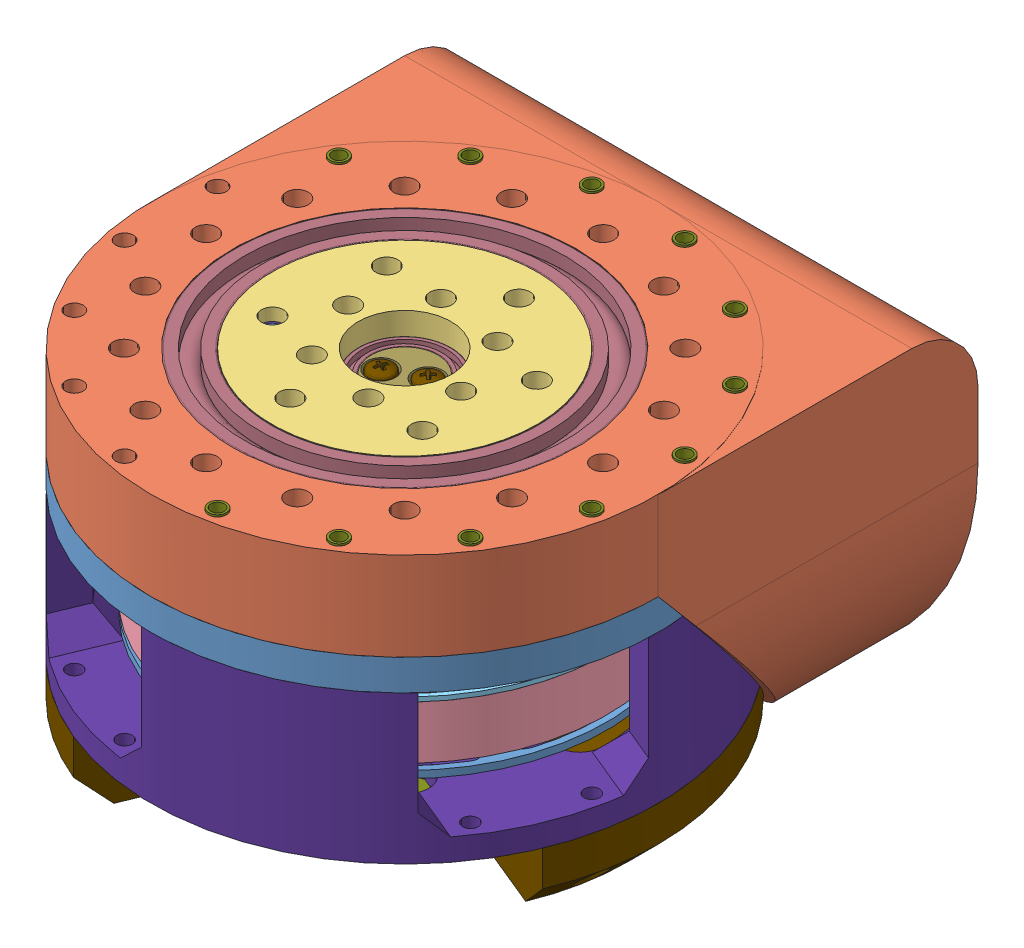
SolidWorks assembly Cycloidal_v3, configuration Default. Lengths in mm.
Overall size (150.25 88 150.25).
347 component instances, 93 part files, 92 mates.
Components (placement in the parent):
- motor-X83008S.stp-1: motor-X83008S.stp [Default] at (86.8737 89.8915 70.5407) x (-0.753247 0 0.657738) z (0 -1 0) size (114.7 114.7 37.62) (hidden)
  - base.stp-1: base.stp [Default] at (42.0794 12.0269 46.7342) size (91.6 91.6 15.61)
  - stator.stp-1: stator.stp [Default] at (42.0794 12.0269 33.1342) x (0.08493 -0.996387 0) z (0 0 1) size (83 83 8)
  - coil.stp-1: coil.stp [Default] at (39.5332 41.8984 37.1342) x (0.996387 0.08493 0) z (-0.08493 0.996387 0) size (4.4 10.2 10.5)
  - coil.stp-2: coil.stp [Default] at (34.3848 41.0025 37.1342) x (0.966502 0.256661 0) z (-0.256661 0.966502 0) size (4.4 10.2 10.5)
  - coil.stp-3: coil.stp [Default] at (29.4701 39.2261 37.1342) x (0.90725 0.420593 0) z (-0.420593 0.90725 0) size (4.4 10.2 10.5)
  - coil.stp-4: coil.stp [Default] at (24.9386 36.6233 37.1342) x (0.820431 0.571745 0) z (-0.571745 0.820431 0) size (4.4 10.2 10.5)
  - coil.stp-5: coil.stp [Default] at (20.9279 33.2732 37.1342) x (0.708685 0.705525 0) z (-0.705525 0.708685 0) size (4.4 10.2 10.5)
  - coil.stp-6: coil.stp [Default] at (17.5599 29.2775 37.1342) x (0.575405 0.817869 0) z (-0.817869 0.575405 0) size (4.4 10.2 10.5)
  - coil.stp-7: coil.stp [Default] at (14.9368 24.7576 37.1342) x (0.424642 0.905361 0) z (-0.905361 0.424642 0) size (4.4 10.2 10.5)
  - coil.stp-8: coil.stp [Default] at (13.1385 19.8509 37.1342) x (0.260976 0.965345 0) z (-0.965345 0.260976 0) size (4.4 10.2 10.5)
  - coil.stp-9: coil.stp [Default] at (12.2196 14.7066 37.1342) x (0.089381 0.995998 0) z (-0.995998 0.089381 0) size (4.4 10.2 10.5)
  - coil.stp-10: coil.stp [Default] at (12.2079 9.4807 37.1342) x (-0.08493 0.996387 0) z (-0.996387 -0.08493 0) size (4.4 10.2 10.5)
  - coil.stp-11: coil.stp [Default] at (13.1039 4.3323 37.1342) x (-0.256661 0.966502 0) z (-0.966502 -0.256661 0) size (4.4 10.2 10.5)
  - coil.stp-12: coil.stp [Default] at (14.8802 -0.5824 37.1342) x (-0.420593 0.90725 0) z (-0.90725 -0.420593 0) size (4.4 10.2 10.5)
  - coil.stp-13: coil.stp [Default] at (17.483 -5.1139 37.1342) x (-0.571745 0.820431 0) z (-0.820431 -0.571745 0) size (4.4 10.2 10.5)
  - coil.stp-14: coil.stp [Default] at (20.8332 -9.1246 37.1342) x (-0.705525 0.708685 0) z (-0.708685 -0.705525 0) size (4.4 10.2 10.5)
  - coil.stp-15: coil.stp [Default] at (24.8289 -12.4926 37.1342) x (-0.817869 0.575405 0) z (-0.575405 -0.817869 0) size (4.4 10.2 10.5)
  - coil.stp-16: coil.stp [Default] at (29.3487 -15.1157 37.1342) x (-0.905361 0.424642 0) z (-0.424642 -0.905361 0) size (4.4 10.2 10.5)
  - coil.stp-17: coil.stp [Default] at (34.2554 -16.914 37.1342) x (-0.965345 0.260976 0) z (-0.260976 -0.965345 0) size (4.4 10.2 10.5)
  - coil.stp-18: coil.stp [Default] at (39.3998 -17.8329 37.1342) x (-0.995998 0.089381 0) z (-0.089381 -0.995998 0) size (4.4 10.2 10.5)
  - coil.stp-19: coil.stp [Default] at (44.6256 -17.8446 37.1342) x (-0.996387 -0.08493 0) z (0.08493 -0.996387 0) size (4.4 10.2 10.5)
  - coil.stp-20: coil.stp [Default] at (49.7741 -16.9486 37.1342) x (-0.966502 -0.256661 0) z (0.256661 -0.966502 0) size (4.4 10.2 10.5)
  - coil.stp-21: coil.stp [Default] at (54.6887 -15.1723 37.1342) x (-0.90725 -0.420593 0) z (0.420593 -0.90725 0) size (4.4 10.2 10.5)
  - coil.stp-22: coil.stp [Default] at (59.2202 -12.5695 37.1342) x (-0.820431 -0.571745 0) z (0.571745 -0.820431 0) size (4.4 10.2 10.5)
  - coil.stp-23: coil.stp [Default] at (63.2309 -9.2193 37.1342) x (-0.708685 -0.705525 0) z (0.705525 -0.708685 0) size (4.4 10.2 10.5)
  - coil.stp-24: coil.stp [Default] at (66.599 -5.2236 37.1342) x (-0.575405 -0.817869 0) z (0.817869 -0.575405 0) size (4.4 10.2 10.5)
  - coil.stp-25: coil.stp [Default] at (69.222 -0.7038 37.1342) x (-0.424642 -0.905361 0) z (0.905361 -0.424642 0) size (4.4 10.2 10.5)
  - coil.stp-26: coil.stp [Default] at (71.0203 4.2029 37.1342) x (-0.260976 -0.965345 0) z (0.965345 -0.260976 0) size (4.4 10.2 10.5)
  - coil.stp-27: coil.stp [Default] at (71.9392 9.3473 37.1342) x (-0.089381 -0.995998 0) z (0.995998 -0.089381 0) size (4.4 10.2 10.5)
  - coil.stp-28: coil.stp [Default] at (71.9509 14.5731 37.1342) x (0.08493 -0.996387 0) z (0.996387 0.08493 0) size (4.4 10.2 10.5)
  - coil.stp-29: coil.stp [Default] at (71.055 19.7216 37.1342) x (0.256661 -0.966502 0) z (0.966502 0.256661 0) size (4.4 10.2 10.5)
  - coil.stp-30: coil.stp [Default] at (69.2786 24.6362 37.1342) x (0.420593 -0.90725 0) z (0.90725 0.420593 0) size (4.4 10.2 10.5)
  - coil.stp-31: coil.stp [Default] at (66.6758 29.1677 37.1342) x (0.571745 -0.820431 0) z (0.820431 0.571745 0) size (4.4 10.2 10.5)
  - coil.stp-32: coil.stp [Default] at (63.3257 33.1785 37.1342) x (0.705525 -0.708685 0) z (0.708685 0.705525 0) size (4.4 10.2 10.5)
  - coil.stp-33: coil.stp [Default] at (59.33 36.5465 37.1342) x (0.817869 -0.575405 0) z (0.575405 0.817869 0) size (4.4 10.2 10.5)
  - coil.stp-34: coil.stp [Default] at (54.8101 39.1695 37.1342) x (0.905361 -0.424642 0) z (0.424642 0.905361 0) size (4.4 10.2 10.5)
  - coil.stp-35: coil.stp [Default] at (49.9034 40.9678 37.1342) x (0.965345 -0.260976 0) z (0.260976 0.965345 0) size (4.4 10.2 10.5)
  - coil.stp-36: coil.stp [Default] at (44.759 41.8868 37.1342) x (0.995998 -0.089381 0) z (0.089381 0.995998 0) size (4.4 10.2 10.5)
  - rotor.stp-1: rotor.stp [Default] at (42.0794 12.0269 42.1342) x (-0.293442 0.955977 0) z (0 0 -1) size (91.8 91.8 12)
  - outrunner.stp-1: outrunner.stp [Default] at (42.0794 12.0269 30.1342) x (-0.254711 0.967017 0) z (-0.967017 -0.254711 0) size (91.8 17.01 91.8)
  - screw-mount.stp-1: screw-mount.stp [Default] at (38.1314 27.0157 27.1342) x (1 0 0) z (0 0 -1) size (7 7 6.5)
  - screw-mount.stp-2: screw-mount.stp [Default] at (27.0906 8.0789 27.1342) x (1 0 0) z (0 0 -1) size (7 7 6.5)
  - screw-mount.stp-3: screw-mount.stp [Default] at (57.0682 15.9749 27.1342) x (1 0 0) z (0 0 -1) size (7 7 6.5)
  - screw-mount.stp-4: screw-mount.stp [Default] at (46.0274 -2.9618 27.1342) x (1 0 0) z (0 0 -1) size (7 7 6.5)
  - 6702ZZ-bearing-15x21x4.stp-1: 6702ZZ-bearing-15x21x4.stp [Default] at (42.0794 12.0269 43.7342) x (1 0 0) z (0 -1 0) size (21 4 21)
  - 6702ZZ-bearing-15x21x4.stp-2: 6702ZZ-bearing-15x21x4.stp [Default] at (42.0794 12.0269 35.1342) x (1 0 0) z (0 1 0) size (21 4 21)
  - shaft.stp-1: shaft.stp [Default] at (42.0794 12.0269 20.1342) size (16 16 31.6)
  - fix-screw.stp-1: fix-screw.stp [Default] at (42.0794 12.0269 51.7342) x (1 0 0) z (0 0 -1) size (19.67 18.96 12.02)
- Base_Plate-1: Base_Plate [Default] at (47.267 69.7573 89.1587) x (0.895936 0 -0.444184) z (0.444184 0 0.895936) size (40 7 40)
- Eccentric_Shaft-1: Eccentric_Shaft [Default] at (38.0321 70.4165 102.2536) x (-0.444184 0 -0.895936) z (0.895936 0 -0.444184) size (20 15 17)
  - Eccentric_Shaft_bot-1: Eccentric_Shaft_bot [Default] at (7.6302 6.3409 14.0904) size (17 5 17)
  - Eccentric_Shaft_bot-2: Eccentric_Shaft_bot [Default] at (7.6302 11.3409 14.0904) x (-1 0 0) z (0 0 -1) size (17 5 17)
  - Eccentric_Shaft_top-1: Eccentric_Shaft_top [Default] at (7.6302 16.3409 14.0904) x (-1 0 0) z (0 0 -1) size (17 5 17)
- radial ball bearing_68_iso-39: radial ball bearing_68_iso [ISO 15 RBB - 1860 - 32,SI,NC,32_68] at (47.267 91.8173 89.1587) x (0 1 0) z (0.105786 0 0.994389) size (10 78 78)
- radial ball bearing_68_iso-40: radial ball bearing_68_iso [ISO 15 RBB - 1840 - 32,SI,NC,32_68] at (47.267 73.2573 89.1587) x (0 1 0) z (-0.019534 0 0.999809) size (7 52 52)
- m13_bearing-31: m13_bearing [Default] at (-10.7414 95.4081 67.0593) x (0.227678 0 0.973736) z (0.973736 0 -0.227678) size (13 16 13)
  - m6-1: m6 [Default] at (8.4921 2.5508 14.8914) size (6 16 6)
  - radial ball bearing_68_iso-1: radial ball bearing_68_iso [ISO 15 RBB - 286 - 10,SI,NC,10_68] at (8.4921 16.0508 14.8914) x (0 1 0) z (0 0 1) size (5 13 13)
  - radial ball bearing_68_iso-2: radial ball bearing_68_iso [ISO 15 RBB - 286 - 10,SI,NC,10_68] at (8.4921 11.0508 14.8914) x (0 1 0) z (0 0 1) size (5 13 13)
- m13_bearing-32: m13_bearing [Default] at (-14.1668 95.4081 84.2801) x (0.227678 0 0.973736) z (0.973736 0 -0.227678) size (13 16 13)
  - m6-1: m6 [Default] at (8.4921 2.5508 14.8914) size (6 16 6)
  - radial ball bearing_68_iso-1: radial ball bearing_68_iso [ISO 15 RBB - 286 - 10,SI,NC,10_68] at (8.4921 16.0508 14.8914) x (0 1 0) z (0 0 1) size (5 13 13)
  - radial ball bearing_68_iso-2: radial ball bearing_68_iso [ISO 15 RBB - 286 - 10,SI,NC,10_68] at (8.4921 11.0508 14.8914) x (0 1 0) z (0 0 1) size (5 13 13)
- m13_bearing-34: m13_bearing [Default] at (13.6125 95.5581 125.8547) x (0.227678 0 0.973736) z (0.973736 0 -0.227678) size (13 16 13)
  - m6-1: m6 [Default] at (8.4921 2.5508 14.8914) size (6 16 6)
  - radial ball bearing_68_iso-1: radial ball bearing_68_iso [ISO 15 RBB - 286 - 10,SI,NC,10_68] at (8.4921 16.0508 14.8914) x (0 1 0) z (0 0 1) size (5 13 13)
  - radial ball bearing_68_iso-2: radial ball bearing_68_iso [ISO 15 RBB - 286 - 10,SI,NC,10_68] at (8.4921 11.0508 14.8914) x (0 1 0) z (0 0 1) size (5 13 13)
- m13_bearing-35: m13_bearing [Default] at (-0.9866 95.4081 116.0999) x (0.227678 0 0.973736) z (0.973736 0 -0.227678) size (13 16 13)
  - m6-1: m6 [Default] at (8.4921 2.5508 14.8914) size (6 16 6)
  - radial ball bearing_68_iso-1: radial ball bearing_68_iso [ISO 15 RBB - 286 - 10,SI,NC,10_68] at (8.4921 16.0508 14.8914) x (0 1 0) z (0 0 1) size (5 13 13)
  - radial ball bearing_68_iso-2: radial ball bearing_68_iso [ISO 15 RBB - 286 - 10,SI,NC,10_68] at (8.4921 11.0508 14.8914) x (0 1 0) z (0 0 1) size (5 13 13)
- m13_bearing-36: m13_bearing [Default] at (-10.7414 95.5581 101.5009) x (0.227678 0 0.973736) z (0.973736 0 -0.227678) size (13 16 13)
  - m6-1: m6 [Default] at (8.4921 2.5508 14.8914) size (6 16 6)
  - radial ball bearing_68_iso-1: radial ball bearing_68_iso [ISO 15 RBB - 286 - 10,SI,NC,10_68] at (8.4921 16.0508 14.8914) x (0 1 0) z (0 0 1) size (5 13 13)
  - radial ball bearing_68_iso-2: radial ball bearing_68_iso [ISO 15 RBB - 286 - 10,SI,NC,10_68] at (8.4921 11.0508 14.8914) x (0 1 0) z (0 0 1) size (5 13 13)
- m13_bearing-1: m13_bearing [Default] at (-0.8801 95.4081 62.5627) x (0.736525 0 0.676411) z (0.676411 0 -0.736525) size (13 16 13)
  - m6-1: m6 [Default] at (8.4921 2.5508 14.8914) size (6 16 6)
  - radial ball bearing_68_iso-1: radial ball bearing_68_iso [ISO 15 RBB - 286 - 10,SI,NC,10_68] at (8.4921 16.0508 14.8914) x (0 1 0) z (0 0 1) size (5 13 13)
  - radial ball bearing_68_iso-2: radial ball bearing_68_iso [ISO 15 RBB - 286 - 10,SI,NC,10_68] at (8.4921 11.0508 14.8914) x (0 1 0) z (0 0 1) size (5 13 13)
- m13_bearing-2: m13_bearing [Default] at (48.6831 95.4081 124.0939) x (0.120271 0 0.992741) z (0.992741 0 -0.120271) size (13 16 13)
  - m6-1: m6 [Default] at (8.4921 2.5508 14.8914) size (6 16 6)
  - radial ball bearing_68_iso-1: radial ball bearing_68_iso [ISO 15 RBB - 286 - 10,SI,NC,10_68] at (8.4921 16.0508 14.8914) x (0 1 0) z (0 0 1) size (5 13 13)
  - radial ball bearing_68_iso-2: radial ball bearing_68_iso [ISO 15 RBB - 286 - 10,SI,NC,10_68] at (8.4921 11.0508 14.8914) x (0 1 0) z (0 0 1) size (5 13 13)
- m13_bearing-3: m13_bearing [Default] at (32.7832 95.4081 34.9886) x (-0.046141 0 0.998935) z (0.998935 0 0.046141) size (13 16 13)
  - m6-1: m6 [Default] at (8.4921 2.5508 14.8914) size (6 16 6)
  - radial ball bearing_68_iso-1: radial ball bearing_68_iso [ISO 15 RBB - 286 - 10,SI,NC,10_68] at (8.4921 16.0508 14.8914) x (0 1 0) z (0 0 1) size (5 13 13)
  - radial ball bearing_68_iso-2: radial ball bearing_68_iso [ISO 15 RBB - 286 - 10,SI,NC,10_68] at (8.4921 11.0508 14.8914) x (0 1 0) z (0 0 1) size (5 13 13)
- m13_bearing-4: m13_bearing [Default] at (77.6928 95.3081 80.133) x (-0.036208 0 0.999344) z (0.999344 0 0.036208) size (13 16 13)
  - m6-1: m6 [Default] at (8.4921 2.5508 14.8914) size (6 16 6)
  - radial ball bearing_68_iso-1: radial ball bearing_68_iso [ISO 15 RBB - 286 - 10,SI,NC,10_68] at (8.4921 16.0508 14.8914) x (0 1 0) z (0 0 1) size (5 13 13)
  - radial ball bearing_68_iso-2: radial ball bearing_68_iso [ISO 15 RBB - 286 - 10,SI,NC,10_68] at (8.4921 11.0508 14.8914) x (0 1 0) z (0 0 1) size (5 13 13)
- m13_bearing-5: m13_bearing [Default] at (73.474 95.4081 98.7828) x (0.059133 0 0.99825) z (0.99825 0 -0.059133) size (13 16 13)
  - m6-1: m6 [Default] at (8.4921 2.5508 14.8914) size (6 16 6)
  - radial ball bearing_68_iso-1: radial ball bearing_68_iso [ISO 15 RBB - 286 - 10,SI,NC,10_68] at (8.4921 16.0508 14.8914) x (0 1 0) z (0 0 1) size (5 13 13)
  - radial ball bearing_68_iso-2: radial ball bearing_68_iso [ISO 15 RBB - 286 - 10,SI,NC,10_68] at (8.4921 11.0508 14.8914) x (0 1 0) z (0 0 1) size (5 13 13)
- m13_bearing-6: m13_bearing [Default] at (12.9248 95.4081 46.7315) x (0.451561 0 0.89224) z (0.89224 0 -0.451561) size (13 16 13)
  - m6-1: m6 [Default] at (8.4921 2.5508 14.8914) size (6 16 6)
  - radial ball bearing_68_iso-1: radial ball bearing_68_iso [ISO 15 RBB - 286 - 10,SI,NC,10_68] at (8.4921 16.0508 14.8914) x (0 1 0) z (0 0 1) size (5 13 13)
  - radial ball bearing_68_iso-2: radial ball bearing_68_iso [ISO 15 RBB - 286 - 10,SI,NC,10_68] at (8.4921 11.0508 14.8914) x (0 1 0) z (0 0 1) size (5 13 13)
- m13_bearing-7: m13_bearing [Default] at (56.6452 95.4081 32.3406) x (-0.545813 0 0.837907) z (0.837907 0 0.545813) size (13 16 13)
  - m6-1: m6 [Default] at (8.4921 2.5508 14.8914) size (6 16 6)
  - radial ball bearing_68_iso-1: radial ball bearing_68_iso [ISO 15 RBB - 286 - 10,SI,NC,10_68] at (8.4921 16.0508 14.8914) x (0 1 0) z (0 0 1) size (5 13 13)
  - radial ball bearing_68_iso-2: radial ball bearing_68_iso [ISO 15 RBB - 286 - 10,SI,NC,10_68] at (8.4921 11.0508 14.8914) x (0 1 0) z (0 0 1) size (5 13 13)
- m13_bearing-8: m13_bearing [Default] at (63.0373 95.4081 51.3153) x (0.158553 0 0.98735) z (0.98735 0 -0.158553) size (13 16 13)
  - m6-1: m6 [Default] at (8.4921 2.5508 14.8914) size (6 16 6)
  - radial ball bearing_68_iso-1: radial ball bearing_68_iso [ISO 15 RBB - 286 - 10,SI,NC,10_68] at (8.4921 16.0508 14.8914) x (0 1 0) z (0 0 1) size (5 13 13)
  - radial ball bearing_68_iso-2: radial ball bearing_68_iso [ISO 15 RBB - 286 - 10,SI,NC,10_68] at (8.4921 11.0508 14.8914) x (0 1 0) z (0 0 1) size (5 13 13)
- m13_bearing-9: m13_bearing [Default] at (83.8577 95.4081 55.5358) x (-0.687134 0 0.72653) z (0.72653 0 0.687134) size (13 16 13)
  - m6-1: m6 [Default] at (8.4921 2.5508 14.8914) size (6 16 6)
  - radial ball bearing_68_iso-1: radial ball bearing_68_iso [ISO 15 RBB - 286 - 10,SI,NC,10_68] at (8.4921 16.0508 14.8914) x (0 1 0) z (0 0 1) size (5 13 13)
  - radial ball bearing_68_iso-2: radial ball bearing_68_iso [ISO 15 RBB - 286 - 10,SI,NC,10_68] at (8.4921 11.0508 14.8914) x (0 1 0) z (0 0 1) size (5 13 13)
- m13_bearing-11: m13_bearing [Default] at (30.1977 95.4081 135.7424) x (0.57351 0 0.819198) z (0.819198 0 -0.57351) size (13 16 13)
  - m6-1: m6 [Default] at (8.4921 2.5508 14.8914) size (6 16 6)
  - radial ball bearing_68_iso-1: radial ball bearing_68_iso [ISO 15 RBB - 286 - 10,SI,NC,10_68] at (8.4921 16.0508 14.8914) x (0 1 0) z (0 0 1) size (5 13 13)
  - radial ball bearing_68_iso-2: radial ball bearing_68_iso [ISO 15 RBB - 286 - 10,SI,NC,10_68] at (8.4921 11.0508 14.8914) x (0 1 0) z (0 0 1) size (5 13 13)
- m13_bearing-12: m13_bearing [Default] at (62.8861 95.4081 115.3744) x (0.184178 0 0.982893) z (0.982893 0 -0.184178) size (13 16 13)
  - m6-1: m6 [Default] at (8.4921 2.5508 14.8914) size (6 16 6)
  - radial ball bearing_68_iso-1: radial ball bearing_68_iso [ISO 15 RBB - 286 - 10,SI,NC,10_68] at (8.4921 16.0508 14.8914) x (0 1 0) z (0 0 1) size (5 13 13)
  - radial ball bearing_68_iso-2: radial ball bearing_68_iso [ISO 15 RBB - 286 - 10,SI,NC,10_68] at (8.4921 11.0508 14.8914) x (0 1 0) z (0 0 1) size (5 13 13)
- socket button head screw_iso-2: socket button head screw_iso [ISO 7380 - M4 x 12 - 12N] at (47.267 67.4573 134.1587) x (0 1 0) z (-0.724148 0 0.689645) size (14.2 7.6 7.6)
- socket button head screw_iso-3: socket button head screw_iso [ISO 7380 - M4 x 12 - 12N] at (15.4472 67.4573 57.3389) x (0 1 0) z (-0.724148 0 0.689645) size (14.2 7.6 7.6)
- socket button head screw_iso-4: socket button head screw_iso [ISO 7380 - M4 x 12 - 12N] at (30.0462 67.4573 47.5841) x (0 1 0) z (-0.724148 0 0.689645) size (14.2 7.6 7.6)
- socket button head screw_iso-5: socket button head screw_iso [ISO 7380 - M4 x 12 - 12N] at (47.267 67.4573 44.1587) x (0 1 0) z (-0.724148 0 0.689645) size (14.2 7.6 7.6)
- socket button head screw_iso-6: socket button head screw_iso [ISO 7380 - M4 x 12 - 12N] at (64.4877 67.4573 47.5841) x (0 1 0) z (-0.724148 0 0.689645) size (14.2 7.6 7.6)
- socket button head screw_iso-8: socket button head screw_iso [ISO 7380 - M4 x 12 - 12N] at (88.8416 67.4573 71.9379) x (0 1 0) z (-0.724148 0 0.689645) size (14.2 7.6 7.6)
- socket button head screw_iso-9: socket button head screw_iso [ISO 7380 - M4 x 12 - 12N] at (92.267 67.4573 89.1587) x (0 1 0) z (-0.724148 0 0.689645) size (14.2 7.6 7.6)
- socket button head screw_iso-10: socket button head screw_iso [ISO 7380 - M4 x 12 - 12N] at (88.8416 67.4573 106.3794) x (0 1 0) z (-0.724148 0 0.689645) size (14.2 7.6 7.6)
- socket button head screw_iso-11: socket button head screw_iso [ISO 7380 - M4 x 12 - 12N] at (79.0868 67.4573 120.9785) x (0 1 0) z (-0.724148 0 0.689645) size (14.2 7.6 7.6)
- M3x4x4.2_brass_insert-2: M3x4x4.2_brass_insert [Default] at (2.3676 97.2573 59.1579) x (-0.680278 0 -0.732954) z (-0.732954 0 0.680278) size (4 4 4)
- M3x4x4.2_brass_insert-3: M3x4x4.2_brass_insert [Default] at (17.2662 97.2573 44.2593) x (-0.509546 0 -0.860444) z (-0.860444 0 0.509546) size (4 4 4)
- M3x4x4.2_brass_insert-6: M3x4x4.2_brass_insert [Default] at (77.2678 97.2573 44.2593) x (-0.680278 0 -0.732954) z (-0.732954 0 0.680278) size (4 4 4)
- M3x4x4.2_brass_insert-8: M3x4x4.2_brass_insert [Default] at (100.2294 93.2573 78.6238) x (-0.970393 0 0.241533) z (-0.241533 0 -0.970393) size (4 4 4)
- M3x4x4.2_brass_insert-14: M3x4x4.2_brass_insert [Default] at (36.7321 97.2573 36.1963) x (0.509546 0 0.860444) z (0.860444 0 -0.509546) size (4 4 4)
- M3x4x4.2_brass_insert-15: M3x4x4.2_brass_insert [Default] at (57.8019 93.2573 36.1963) x (0.897191 0 -0.441644) z (0.441644 0 0.897191) size (4 4 4)
- M3x4x4.2_brass_insert-16: M3x4x4.2_brass_insert [Default] at (92.1663 97.2573 59.1579) x (-0.680278 0 -0.732954) z (-0.732954 0 0.680278) size (4 4 4)
- M3x4x4.2_brass_insert-17: M3x4x4.2_brass_insert [Default] at (100.2294 97.2573 99.6935) x (0.680278 0 0.732954) z (0.732954 0 -0.680278) size (4 4 4)
- M3x4x4.2_brass_insert-19: M3x4x4.2_brass_insert [Default] at (92.1663 97.2573 119.1595) x (0.680278 0 0.732954) z (0.732954 0 -0.680278) size (4 4 4)
- M3x4x4.2_brass_insert-20: M3x4x4.2_brass_insert [Default] at (77.2678 97.2573 134.058) x (0.680278 0 0.732954) z (0.732954 0 -0.680278) size (4 4 4)
- M3x4x4.2_brass_insert-21: M3x4x4.2_brass_insert [Default] at (57.8019 97.2573 142.1211) x (0.680278 0 0.732954) z (0.732954 0 -0.680278) size (4 4 4)
- M4x6x5.5_brass_insert-47: M4x6x5.5_brass_insert [Default] at (5.6924 92.8573 71.9379) x (0.474598 0 0.880203) z (0 1 0) size (5 5 6)
- M4x6x5.5_brass_insert-48: M4x6x5.5_brass_insert [Default] at (2.267 92.8573 89.1587) x (0.260051 0 0.965595) z (0 1 0) size (5 5 6)
- M4x6x5.5_brass_insert-49: M4x6x5.5_brass_insert [Default] at (5.6924 87.0073 106.3794) x (-0.745833 0 0.666133) z (0 -1 0) size (5 5 6)
- M4x6x5.5_brass_insert-50: M4x6x5.5_brass_insert [Default] at (15.4472 86.8573 120.9785) x (-0.745833 0 0.666133) z (0 -1 0) size (5 5 6)
- M4x6x5.5_brass_insert-51: M4x6x5.5_brass_insert [Default] at (30.0462 87.0073 130.7332) x (0.260051 0 -0.965595) z (0 -1 0) size (5 5 6)
- M4x6x5.5_brass_insert-6: M4x6x5.5_brass_insert [Default] at (25.9649 93.9895 97.8316) x (0.252509 0 0.967595) z (0 1 0) size (5 5 6)
- M4x6x5.5_brass_insert-20: M4x6x5.5_brass_insert [Default] at (64.4877 86.8573 130.7332) x (-0.745833 0 0.666133) z (0 -1 0) size (5 5 6)
- M4x6x5.5_brass_insert-21: M4x6x5.5_brass_insert [Default] at (47.267 86.8573 134.1587) x (-0.745833 0 0.666133) z (0 -1 0) size (5 5 6)
- M4x6x5.5_brass_insert-22: M4x6x5.5_brass_insert [Default] at (15.4472 86.8573 57.3389) x (0.623293 0 0.781988) z (0 -1 0) size (5 5 6)
- M4x6x5.5_brass_insert-23: M4x6x5.5_brass_insert [Default] at (30.0462 86.8573 47.5841) x (0.623293 0 0.781988) z (0 -1 0) size (5 5 6)
- M4x6x5.5_brass_insert-24: M4x6x5.5_brass_insert [Default] at (79.0868 86.8573 120.9785) x (0.541965 0 0.840401) z (0 -1 0) size (5 5 6)
- M4x6x5.5_brass_insert-25: M4x6x5.5_brass_insert [Default] at (88.8416 86.8573 106.3794) x (-0.745833 0 0.666133) z (0 -1 0) size (5 5 6)
- M4x6x5.5_brass_insert-26: M4x6x5.5_brass_insert [Default] at (92.267 86.8573 89.1587) x (-0.745833 0 0.666133) z (0 -1 0) size (5 5 6)
- M4x6x5.5_brass_insert-27: M4x6x5.5_brass_insert [Default] at (88.8416 86.8573 71.9379) x (-0.745833 0 0.666133) z (0 -1 0) size (5 5 6)
- M4x6x5.5_brass_insert-28: M4x6x5.5_brass_insert [Default] at (79.0868 92.8573 57.3389) x (0.260051 0 0.965595) z (0 1 0) size (5 5 6)
- M4x6x5.5_brass_insert-29: M4x6x5.5_brass_insert [Default] at (64.4877 86.8573 47.5841) x (-0.142939 0 0.989731) z (0 -1 0) size (5 5 6)
- M4x6x5.5_brass_insert-31: M4x6x5.5_brass_insert [Default] at (47.267 86.8573 44.1587) x (-0.220341 0 0.975423) z (0 -1 0) size (5 5 6)
- pan cross head_am-1: pan cross head_am [B18.6.7M - M3 x 0.5 x 20 Type I Cross Recessed PHMS --20N] at (50.8507 92.6573 87.3819) x (0 -1 0) z (0.748822 0 0.662771) size (22.37 5.6 5.6)
- pan cross head_am-3: pan cross head_am [B18.6.7M - M3 x 0.5 x 20 Type I Cross Recessed PHMS --20N] at (43.6832 92.6573 90.9354) x (0 -1 0) z (0.940321 0 0.340288) size (22.37 5.6 5.6)
- M3x4x4.2_brass_insert-22: M3x4x4.2_brass_insert [Default] at (50.8507 69.7573 87.3819) x (0.984485 0 -0.175469) z (0.175469 0 0.984485) size (4 4 4)
- M3x4x4.2_brass_insert-23: M3x4x4.2_brass_insert [Default] at (43.6832 69.7573 90.9354) x (0.984609 0 -0.174769) z (0.174769 0 0.984609) size (4 4 4)
- pan cross head_am-4: pan cross head_am [B18.6.7M - M3 x 0.5 x 10 Type I Cross Recessed PHMS --10N] at (33.38 77.6573 96.0435) x (0 -1 0) z (0 0 1) size (12.37 5.6 5.6)
- pan cross head_am-5: pan cross head_am [B18.6.7M - M3 x 0.5 x 10 Type I Cross Recessed PHMS --10N] at (61.154 77.6573 82.2738) x (0 -1 0) z (0 0 1) size (12.37 5.6 5.6)
- pan cross head_am-6: pan cross head_am [B18.6.7M - M3 x 0.5 x 10 Type I Cross Recessed PHMS --10N] at (54.1518 77.6573 103.0457) x (0 -1 0) z (0 0 1) size (12.37 5.6 5.6)
- pan cross head_am-7: pan cross head_am [B18.6.7M - M3 x 0.5 x 10 Type I Cross Recessed PHMS --10N] at (40.3821 77.6573 75.2717) x (0 -1 0) z (0 0 1) size (12.37 5.6 5.6)
- radial ball bearing_68_iso-44: radial ball bearing_68_iso [ISO 15 RBB - 1715 - 26,SI,NC,26_68] at (46.6007 84.7573 87.8148) x (0 1 0) z (-0.714953 0 -0.699173) size (4 21 21)
- radial ball bearing_68_iso-45: radial ball bearing_68_iso [ISO 15 RBB - 1715 - 26,SI,NC,26_68] at (47.267 89.7573 89.1587) x (0 1 0) z (0.999483 0 -0.032163) size (4 21 21)
- radial ball bearing_68_iso-46: radial ball bearing_68_iso [ISO 15 RBB - 1715 - 26,SI,NC,26_68] at (47.9333 79.7573 90.5026) x (0 1 0) z (0.000644 0 1) size (4 21 21)
- socket button head screw_iso-37: socket button head screw_iso [ISO 7380 - M4 x 12 - 12N] at (79.0868 67.4573 57.3389) x (0 1 0) z (-0.709975 0 0.704227) size (14.2 7.6 7.6)
- socket button head screw_iso-38: socket button head screw_iso [ISO 7380 - M4 x 12 - 12N] at (64.4877 67.4573 130.7332) x (0 1 0) z (-0.724148 0 0.689645) size (14.2 7.6 7.6)
- foc-motor-controller.step-1: foc-motor-controller.step [Default] at (47.267 33.7573 89.1587) x (-0.382683 0 -0.92388) z (0 -1 0) size (57.23 50 8.13)
  - RTA0040B.step-1: RTA0040B.step [Default] at (12.5014 -1.6986 1.595) x (-0.707107 -0.707107 0) z (0 0 1) size (6 6 1)
    - FRAME.step-1: FRAME.step [Default] x (1 0 0) z (0 -1 0) size (6 0.2 6)
      - SOLID.step-1: SOLID.step [Default] at origin size (0.4 0.2 0.22)
      - SOLID-0.step-1: SOLID-0.step [Default] at origin size (0.4 0.2 0.22)
      - SOLID-1.step-1: SOLID-1.step [Default] at origin size (0.4 0.2 0.22)
      - SOLID-2.step-1: SOLID-2.step [Default] at origin size (0.4 0.2 0.22)
      - SOLID-3.step-1: SOLID-3.step [Default] at origin size (0.4 0.2 0.22)
      - SOLID-4.step-1: SOLID-4.step [Default] at origin size (0.4 0.2 0.22)
      - SOLID-5.step-1: SOLID-5.step [Default] at origin size (0.4 0.2 0.22)
      - SOLID-6.step-1: SOLID-6.step [Default] at origin size (0.4 0.2 0.22)
      - SOLID-7.step-1: SOLID-7.step [Default] at origin size (0.4 0.2 0.22)
      - SOLID-8.step-1: SOLID-8.step [Default] at origin size (0.4 0.2 0.22)
      - SOLID-9.step-1: SOLID-9.step [Default] at origin size (0.22 0.2 0.4)
      - SOLID-10.step-1: SOLID-10.step [Default] at origin size (0.22 0.2 0.4)
      - SOLID-11.step-1: SOLID-11.step [Default] at origin size (0.22 0.2 0.4)
      - SOLID-12.step-1: SOLID-12.step [Default] at origin size (0.22 0.2 0.4)
      - SOLID-13.step-1: SOLID-13.step [Default] at origin size (0.22 0.2 0.4)
      - SOLID-14.step-1: SOLID-14.step [Default] at origin size (0.22 0.2 0.4)
      - SOLID-15.step-1: SOLID-15.step [Default] at origin size (0.22 0.2 0.4)
      - SOLID-16.step-1: SOLID-16.step [Default] at origin size (0.22 0.2 0.4)
      - SOLID-17.step-1: SOLID-17.step [Default] at origin size (4.15 0.2 4.15)
      - SOLID-18.step-1: SOLID-18.step [Default] at origin size (0.28 0.1 0.28)
      - SOLID-19.step-1: SOLID-19.step [Default] at origin size (0.28 0.1 0.28)
      - SOLID-20.step-1: SOLID-20.step [Default] at origin size (0.28 0.1 0.28)
      - SOLID-21.step-1: SOLID-21.step [Default] at origin size (0.28 0.1 0.28)
      - SOLID-22.step-1: SOLID-22.step [Default] at origin size (0.4 0.2 0.22)
      - SOLID-23.step-1: SOLID-23.step [Default] at origin size (0.4 0.2 0.22)
      - SOLID-24.step-1: SOLID-24.step [Default] at origin size (0.4 0.2 0.22)
      - SOLID-25.step-1: SOLID-25.step [Default] at origin size (0.4 0.2 0.22)
      - SOLID-26.step-1: SOLID-26.step [Default] at origin size (0.4 0.2 0.22)
      - SOLID-27.step-1: SOLID-27.step [Default] at origin size (0.4 0.2 0.22)
      - SOLID-28.step-1: SOLID-28.step [Default] at origin size (0.4 0.2 0.22)
      - SOLID-29.step-1: SOLID-29.step [Default] at origin size (0.4 0.2 0.22)
      - SOLID-30.step-1: SOLID-30.step [Default] at origin size (0.4 0.2 0.22)
      - SOLID-31.step-1: SOLID-31.step [Default] at origin size (0.4 0.2 0.22)
      - SOLID-32.step-1: SOLID-32.step [Default] at origin size (0.22 0.2 0.4)
      - SOLID-33.step-1: SOLID-33.step [Default] at origin size (0.22 0.2 0.4)
      - SOLID-34.step-1: SOLID-34.step [Default] at origin size (0.22 0.2 0.4)
      - SOLID-35.step-1: SOLID-35.step [Default] at origin size (0.22 0.2 0.4)
      - SOLID-36.step-1: SOLID-36.step [Default] at origin size (0.22 0.2 0.4)
      - SOLID-37.step-1: SOLID-37.step [Default] at origin size (0.22 0.2 0.4)
      - SOLID-38.step-1: SOLID-38.step [Default] at origin size (0.22 0.2 0.4)
      - SOLID-39.step-1: SOLID-39.step [Default] at origin size (0.22 0.2 0.4)
      - SOLID-40.step-1: SOLID-40.step [Default] at origin size (0.22 0.2 0.4)
      - SOLID-41.step-1: SOLID-41.step [Default] at origin size (0.22 0.2 0.4)
      - SOLID-42.step-1: SOLID-42.step [Default] at origin size (0.22 0.2 0.4)
      - SOLID-43.step-1: SOLID-43.step [Default] at origin size (0.22 0.2 0.4)
    - BODY.step-1: BODY.step [Default] at (0 0 0.025) x (1 0 0) z (0 -1 0) size (6 0.97 6)
  - Resonator_SMD_Murata_CSTxExxV-3Pin_3.0x1.1mm.step-1: Resonator_SMD_Murata_CSTxExxV-3Pin_3.0x1.1mm.step [Default] at (1.8 -7 1.595) x (0 1 0) z (0 0 1) size (3.2 1.35 0.9)
  - C_0603_1608Metric.step-1: C_0603_1608Metric.step [Default] at (6.2 -16.8 1.595) x (0 -1 0) z (0 0 1) size (1.6 0.8 0.8)
  - R_0603_1608Metric.step-1: R_0603_1608Metric.step [Default] at (11.8 -7.375 1.595) x (0 1 0) z (0 0 1) size (1.6 0.8 0.45)
  - R_0603_1608Metric.step-2: R_0603_1608Metric.step [Default] at (13.8 -16.8 1.595) x (0 1 0) z (0 0 1) size (1.6 0.8 0.45)
  - R_0603_1608Metric.step-3: R_0603_1608Metric.step [Default] at (18.1 -5.36 1.595) size (1.6 0.8 0.45)
  - C_0603_1608Metric.step-2: C_0603_1608Metric.step [Default] at (2.6 -0.5 1.595) x (0 -1 0) z (0 0 1) size (1.6 0.8 0.8)
  - R_0603_1608Metric.step-4: R_0603_1608Metric.step [Default] at (14.6 -11.3 1.595) x (0 1 0) z (0 0 1) size (1.6 0.8 0.45)
  - L_APV_ANR4020.step-1: L_APV_ANR4020.step [Default] at (22.3 -13.7 1.595) x (0 -1 0) z (0 0 1) size (4.02 4 2)
  - C_0603_1608Metric.step-3: C_0603_1608Metric.step [Default] at (0.3 -12.6 1.595) x (-1 0 0) z (0 0 1) size (1.6 0.8 0.8)
  - C_1206_3216Metric.step-1: C_1206_3216Metric.step [Default] at (15.7 11 1.595) x (0 1 0) z (0 0 1) size (3.2 1.6 1.6)
  - C_0603_1608Metric.step-4: C_0603_1608Metric.step [Default] at (0.3 -9.6 1.595) size (1.6 0.8 0.8)
  - R_0603_1608Metric.step-5: R_0603_1608Metric.step [Default] at (12.3 -16.8 1.595) x (0 1 0) z (0 0 1) size (1.6 0.8 0.45)
  - C_0603_1608Metric.step-5: C_0603_1608Metric.step [Default] at (-0.3 -16.6 1.595) x (0 1 0) z (0 0 1) size (1.6 0.8 0.8)
  - R_0603_1608Metric.step-6: R_0603_1608Metric.step [Default] at (10.9 4.1 1.595) size (1.6 0.8 0.45)
  - C_1206_3216Metric.step-2: C_1206_3216Metric.step [Default] at (6.3 11 1.595) x (0 1 0) z (0 0 1) size (3.2 1.6 1.6)
  - XT30PW_2_2_-M.G.B.step-1: XT30PW_2_2_-M.G.B.step [Default] at (-20.5 9.5 1.595) x (0 -1 0) z (-1 0 0) size (15.5 7.1 12.53)
  - R_0603_1608Metric.step-7: R_0603_1608Metric.step [Default] at (0.3 -11.1 1.595) size (1.6 0.8 0.45)
  - C_0603_1608Metric.step-6: C_0603_1608Metric.step [Default] at (19 -0.4 1.595) x (-0.707107 -0.707107 0) z (0 0 1) size (1.6 0.8 0.8)
  - C_1206_3216Metric.step-3: C_1206_3216Metric.step [Default] at (13.3 11 1.595) x (0 1 0) z (0 0 1) size (3.2 1.6 1.6)
  - R_0603_1608Metric.step-8: R_0603_1608Metric.step [Default] at (10.2 -7.375 1.595) x (0 -1 0) z (0 0 1) size (1.6 0.8 0.45)
  - JST_GH_SM08B-GHS-TB_1x08-1MP_P1.25mm_Horizontal.step-1: JST_GH_SM08B-GHS-TB_1x08-1MP_P1.25mm_Horizontal.step [Default] at (10 -22 1.595) size (13.25 4.95 4.25)
  - C_1206_3216Metric.step-4: C_1206_3216Metric.step [Default] at (-12.3 11 1.595) x (0 1 0) z (0 0 1) size (3.2 1.6 1.6)
  - JST_GH_SM06B-GHS-TB_1x06-1MP_P1.25mm_Horizontal.step-1: JST_GH_SM06B-GHS-TB_1x06-1MP_P1.25mm_Horizontal.step [Default] at (-4.3 -22 1.595) size (10.75 4.95 4.25)
  - C_0603_1608Metric.step-7: C_0603_1608Metric.step [Default] at (7.3 -4.5 1.595) x (-1 0 0) z (0 0 1) size (1.6 0.8 0.8)
  - R_0603_1608Metric.step-9: R_0603_1608Metric.step [Default] at (18.1 -3.86 1.595) x (-1 0 0) z (0 0 1) size (1.6 0.8 0.45)
  - C_1206_3216Metric.step-5: C_1206_3216Metric.step [Default] at (22.6794 -1.2206 1.595) x (0.707107 -0.707107 0) z (0 0 1) size (3.2 1.6 1.6)
  - R_Array_Convex_4x0402.step-1: R_Array_Convex_4x0402.step [Default] at (6.8 -2.5 1.595) size (1 2 0.35)
  - R_0603_1608Metric.step-10: R_0603_1608Metric.step [Default] at (7.7 -16.8 1.595) x (0 -1 0) z (0 0 1) size (1.6 0.8 0.45)
  - C_1206_3216Metric.step-6: C_1206_3216Metric.step [Default] at (8.7 11 1.595) x (0 1 0) z (0 0 1) size (3.2 1.6 1.6)
  - C_0603_1608Metric.step-8: C_0603_1608Metric.step [Default] at (16.1 -11.3 1.595) x (0 1 0) z (0 0 1) size (1.6 0.8 0.8)
  - SOT-23-5.step-1: SOT-23-5.step [Default] at (-3.1 -16.6 1.595) x (-1 0 0) z (0 0 1) size (2.8 2.9 1.55)
  - C_0603_1608Metric.step-9: C_0603_1608Metric.step [Default] at (17.8 -13.6 1.595) size (1.6 0.8 0.8)
  - R_0603_1608Metric.step-11: R_0603_1608Metric.step [Default] at (-11.5 -20.3875 1.595) x (0 -1 0) z (0 0 1) size (1.6 0.8 0.45)
  - C_0603_1608Metric.step-10: C_0603_1608Metric.step [Default] at (-12.4 2.3 1.595) x (0 1 0) z (0 0 1) size (1.6 0.8 0.8)
  - C_1206_3216Metric.step-7: C_1206_3216Metric.step [Default] at (18 11 1.595) x (0 1 0) z (0 0 1) size (3.2 1.6 1.6)
  - R_0603_1608Metric.step-12: R_0603_1608Metric.step [Default] at (-10.8105 -14.9971 1.595) x (-1 0 0) z (0 0 1) size (1.6 0.8 0.45)
  - C_0603_1608Metric.step-11: C_0603_1608Metric.step [Default] at (-13.8 -9.4 1.595) x (-1 0 0) z (0 0 1) size (1.6 0.8 0.8)
  - R_0603_1608Metric.step-13: R_0603_1608Metric.step [Default] at (-23.15 -14.5 1.595) x (-1 0 0) z (0 0 1) size (1.6 0.8 0.45)
  - C_0603_1608Metric.step-12: C_0603_1608Metric.step [Default] at (1.1 -0.2 1.595) x (0 1 0) z (0 0 1) size (1.6 0.8 0.8)
  - D_0805_2012Metric.step-1: D_0805_2012Metric.step [Default] at (22.9 -9.6 1.595) x (0 1 0) z (0 0 1) size (2 1.27 0.8)
  - C_0603_1608Metric.step-13: C_0603_1608Metric.step [Default] at (-7.8 3.775 1.595) x (0 -1 0) z (0 0 1) size (1.6 0.8 0.8)
  - R_0603_1608Metric.step-14: R_0603_1608Metric.step [Default] at (-6.4 -12.825 1.595) x (0 1 0) z (0 0 1) size (1.6 0.8 0.45)
  - L_0603_1608Metric.step-1: L_0603_1608Metric.step [Default] at (-10.1 3 1.595) size (1.6 0.8 0.8)
  - C_0603_1608Metric.step-14: C_0603_1608Metric.step [Default] at (17.9 0.7 1.595) x (-0.707107 -0.707107 0) z (0 0 1) size (1.6 0.8 0.8)
  - HVSSOP-10.step-1: HVSSOP-10.step [Default] at (18.6 -9.6 1.595) x (0 -1 0) z (-1 0 0) size (4.9 1.1 3)
  - C_0603_1608Metric.step-15: C_0603_1608Metric.step [Default] at (7.9 4.1 1.595) x (-1 0 0) z (0 0 1) size (1.6 0.8 0.8)
  - C_0603_1608Metric.step-16: C_0603_1608Metric.step [Default] at (21.1 -9.6 1.595) x (0 -1 0) z (0 0 1) size (1.6 0.8 0.8)
  - R_0603_1608Metric.step-15: R_0603_1608Metric.step [Default] at (-10.8105 -11.9971 1.595) x (-1 0 0) z (0 0 1) size (1.6 0.8 0.45)
  - R_0603_1608Metric.step-16: R_0603_1608Metric.step [Default] at (-18.2 -17.4 1.595) size (1.6 0.8 0.45)
  - C_1206_3216Metric.step-8: C_1206_3216Metric.step [Default] at (-3 11 1.595) x (0 1 0) z (0 0 1) size (3.2 1.6 1.6)
  - R_0603_1608Metric.step-17: R_0603_1608Metric.step [Default] at (-16.9 -20.4 1.595) x (0 -1 0) z (0 0 1) size (1.6 0.8 0.45)
  - R_0603_1608Metric.step-18: R_0603_1608Metric.step [Default] at (-13.3 -20.3875 1.595) x (0 -1 0) z (0 0 1) size (1.6 0.8 0.45)
  - R_0603_1608Metric.step-19: R_0603_1608Metric.step [Default] at (-15.1 -20.3875 1.595) x (0 -1 0) z (0 0 1) size (1.6 0.8 0.45)
  - C_0603_1608Metric.step-17: C_0603_1608Metric.step [Default] at (15.5 -14.4 1.595) x (0 -1 0) z (0 0 1) size (1.6 0.8 0.8)
  - LED_0603_1608Metric.step-1: LED_0603_1608Metric.step [Default] at (-11.5 -23.3875 1.595) x (0 1 0) z (0 0 1) size (1.6 0.8 1.1)
  - C_0805_2012Metric.step-1: C_0805_2012Metric.step [Default] at (19.95 -17 1.595) size (2 1.25 1.25)
  - D_SMB.step-1: D_SMB.step [Default] at (-16.5 11.208 1.595) x (0 -1 0) z (0 0 1) size (5.3 3.55 2.15)
  - C_1206_3216Metric.step-9: C_1206_3216Metric.step [Default] at (-5.3 11 1.595) x (0 1 0) z (0 0 1) size (3.2 1.6 1.6)
  - XT30PW_2_2_-M.G.B.step-2: XT30PW_2_2_-M.G.B.step [Default] at (-20.5 -6.5 1.595) x (0 -1 0) z (-1 0 0) size (15.5 7.1 12.53)
  - C_1206_3216Metric.step-10: C_1206_3216Metric.step [Default] at (1.7 11 1.595) x (0 1 0) z (0 0 1) size (3.2 1.6 1.6)
  - C_1206_3216Metric.step-11: C_1206_3216Metric.step [Default] at (11 11 1.595) x (0 1 0) z (0 0 1) size (3.2 1.6 1.6)
  - C_0603_1608Metric.step-18: C_0603_1608Metric.step [Default] at (-6.3 3.775 1.595) x (0 -1 0) z (0 0 1) size (1.6 0.8 0.8)
  - C_0603_1608Metric.step-19: C_0603_1608Metric.step [Default] at (16.8686 1.7314 1.595) x (0.707107 0.707107 0) z (0 0 1) size (1.6 0.8 0.8)
  - C_0603_1608Metric.step-20: C_0603_1608Metric.step [Default] at (-15.0105 -11.1 1.595) size (1.6 0.8 0.8)
  - C_1206_3216Metric.step-12: C_1206_3216Metric.step [Default] at (-7.7 11 1.595) x (0 1 0) z (0 0 1) size (3.2 1.6 1.6)
  - C_0603_1608Metric.step-21: C_0603_1608Metric.step [Default] at (-18.2 -15.8 1.595) size (1.6 0.8 0.8)
  - C_0603_1608Metric.step-22: C_0603_1608Metric.step [Default] at (-2.1 -11.3 1.595) x (0 -1 0) z (0 0 1) size (1.6 0.8 0.8)
  - C_0603_1608Metric.step-23: C_0603_1608Metric.step [Default] at (-10.8105 -13.4971 1.595) size (1.6 0.8 0.8)
  - C_1206_3216Metric.step-13: C_1206_3216Metric.step [Default] at (4 11 1.595) x (0 1 0) z (0 0 1) size (3.2 1.6 1.6)
